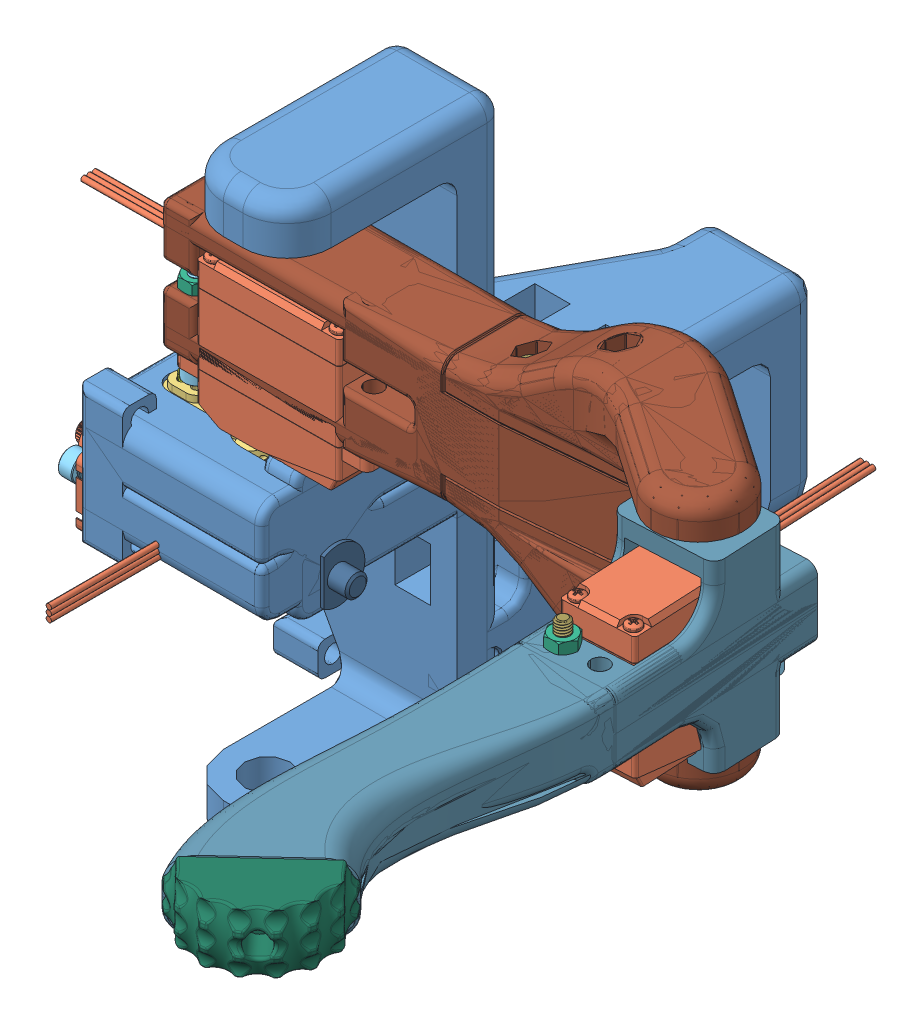
SolidWorks assembly Jambe_gauche, configuration Default. Lengths in mm.
Overall size (226.75 105.95 225.72).
41 component instances, 15 part files, 4 mates.
Components (placement in the parent):
- Hanche-1: Hanche [Default] at origin size (77.1 102.9 99.1)
  - Hanche_V3-1: Hanche_V3 [Default] at origin size (51.8 165 157.2)
  - Servo_DS3225MG-1: Servo_DS3225MG [Default] at (-27.6 -10.2 0) x (0 0 -1) z (-1 0 0) size (87.25 20.4 45.91)
  - Servo_helice-1: Servo_helice [Défaut] at (24 10 0) x (-1 0 0) z (0 -1 0) size (35.39 15.87 6)
  - bearing_535198-1: bearing_535198 [Défaut] at (24 72.6322 0) x (-0.923922 0 -0.382581) z (-0.382581 0 0.923922) size (13.87 4.75 13.87)
  - M4x25mm-1: M4x25mm [91290A176] at (12 -5.2 14.8) x (0 -0.924225 -0.381849) z (1 0 0) size (7 7 29.41)
  - M4x25mm-2: M4x25mm [91290A176] at (12 -15.2 -34.8) x (0 -0.924225 -0.381849) z (1 0 0) size (7 7 29.41)
  - M4_nut-1: M4_nut [90592A090] at (4.3 -15.2 -34.8) x (0 0.866025 0.5) z (0 -0.5 0.866025) size (7 3.75 8.08)
  - M4_nut-2: M4_nut [90592A090] at (4.3 -5.2 14.8) x (0 -0.866025 0.5) z (0 0.5 0.866025) size (7 3.75 8.08)
  - M2x16mm-1: M2x16mm [91290A047] at (24 19 0) x (1 0 0) z (0 1 0) size (3.8 3.8 18.16)
  - M2x16mm-2: M2x16mm [91290A047] at (0 18.4 0) x (1 0 0) z (0 1 0) size (3.8 3.8 18.16)
  - M3x30mm-1: M3x30mm [91290A171] at (29.5 33 -42.25) x (1 0 0) z (0 1 0) size (5.5 5.5 33.33)
  - M3x30mm-2: M3x30mm [91290A171] at (9.5 33 -42.25) x (1 0 0) z (0 1 0) size (5.5 5.5 33.33)
  - M3_nut-1: M3_nut [90592A085] at (29.5 26.2 -42.25) x (0.866025 0 -0.5) z (0.5 0 0.866025) size (5.5 2.79 6.35)
  - M3_nut-2: M3_nut [90592A085] at (9.5 26.2 -42.25) x (0.866025 0 -0.5) z (0.5 0 0.866025) size (5.5 2.79 6.35)
  - Cylinde_bearing-1: Cylinde_bearing [Default] at (37.5 -10.2 0) x (0 -1 0) z (1 0 0) size (15 11.5 12)
- Femur-1: Femur [Default] at (24 49.05 0) x (0 1 0) z (0.999976 0 -0.006973) size (73 46.33 202.15)
  - Femur_V3-1: Femur_V3 [Default] at origin size (73 46.33 172.05)
  - Servo_DS3225MG-1: Servo_DS3225MG [Default] at (-36.05 0 0) x (0 0 1) z (-1 0 0) size (87.25 20.4 45.91)
  - M4x25mm-1: M4x25mm [91290A176] at (3.55 5 -14.8) x (0 -0.070308 -0.997525) z (1 0 0) size (7 7 29.41)
  - M4x25mm-2: M4x25mm [91290A176] at (3.55 -5 34.8) x (0 -0.99819 0.060141) z (1 0 0) size (7 7 29.41)
  - M4_nut-1: M4_nut [90592A090] at (-1.65 5 -14.8) x (0 0.5 0.866025) z (0 -0.866025 0.5) size (7 3.75 8.08)
  - M4_nut-2: M4_nut [90592A090] at (-1.65 -5 34.8) x (0 1 0) z (0 0 1) size (7 3.75 8.08)
  - M4x30mm-1: M4x30mm [91290A180] at (-17 -2.3 71.7972) x (0 0 1) z (-1 0 0) size (7 7 34.38)
  - M4x30mm-2: M4x30mm [91290A180] at (-17 -2.3 96.7972) x (0 0 1) z (-1 0 0) size (7 7 34.38)
  - M4_nut-3: M4_nut [90592A090] at (-14.6 -2.3 71.7972) x (0 0.5 0.866025) z (0 -0.866025 0.5) size (7 3.75 8.08)
  - M4_nut-4: M4_nut [90592A090] at (-14.6 -2.3 96.7972) x (0 1 0) z (0 0 1) size (7 3.75 8.08)
  - Servo_helice-1: Servo_helice [Défaut] at (-32.5 18.86 139.55) x (0 -0.573576 -0.819152) z (-1 0 0) size (35.39 15.87 6)
  - M2_8-1: M2_8 [91292A012] at (-25.5 5.0942 119.8904) x (0 0.030232 -0.999543) z (1 0 0) size (4.5 4.5 10.65)
  - M2_8-2: M2_8 [91292A012] at (-25.5 18.86 139.55) x (0 0.030232 -0.999543) z (1 0 0) size (4.5 4.5 10.65)
  - Cylinde_bearing-1: Cylinde_bearing [Default] at (12.75 0 0) x (0 0 1) z (1 0 0) size (15 11.5 12)
- Tibia-1: Tibia [Default] at (163.6781 57.4324 17.8865) x (0.047809 0 0.998857) z (0.998857 0 -0.047809) size (207.93 61.42 52.63)
  - Tibia_V3-1: Tibia_V3 [Default] at origin size (162.76 52 39.97)
  - Embout_TPE_V3-1: Embout_TPE_V3 [Default] at (129.9518 8.3 0.0575) x (0 -1 0) z (0.642788 0 -0.766044) size (17.12 19.75 39.79)
  - Servo_DS3225MG-1: Servo_DS3225MG [Default] at (0 37.8 0) x (1 0 0) z (0 1 0) size (87.25 20.4 45.91)
  - bearing_535198-1: bearing_535198 [Défaut] at (0 -12.3678 0) x (0.863205 0 0.504854) z (0.504854 0 -0.863205) size (13.87 4.75 13.87)
  - Cylinde_bearing-1: Cylinde_bearing [Default] at (0 -11.6176 0) x (-0.99451 0 0.104639) z (0 -1 0) size (15 11.5 12)
  - M4x25mm-1: M4x25mm [91290A176] at (-14.8 -1.8 5) x (-0.837169 0 -0.546944) z (0 -1 0) size (7 7 29.41)
  - M4x30mm-1: M4x30mm [91290A180] at (34.8 -6.8 -5) x (-0.837169 0 -0.546944) z (0 -1 0) size (7 7 34.38)
  - M4_nut-1: M4_nut [90592A090] at (-14.8 3.4 5) x (0.5 0 0.866025) z (-0.866025 0 0.5) size (7 3.75 8.08)
  - M4_nut-2: M4_nut [90592A090] at (34.8 -1.6 -5) size (7 3.75 8.08)
Mates (geometry in assembly coordinates):
- Concentric1: concentric aligned: cylinder of Hanche-1/bearing_535198-1 through (24 72.6322 0) axis (0 -1 0) radius 3.175; cylinder of Femur-1/Femur_V3-1 through (24 59.8 0) axis (0 -1 0) radius 3.15
- Distance1: distance = 1 mm anti-aligned: plane of Hanche-1/Servo_helice-1 through (24 16 0) normal (0 1 0); plane of Femur-1/Servo_DS3225MG-1 through (24 17 0) normal (0 -1 0)
- Concentric2: concentric aligned: cylinder of Femur-1/Femur_V3-1 through (163.6781 83.05 17.8865) axis (0 -1 0) radius 3.15; cylinder of Tibia-1/Cylinde_bearing-1 through (163.6781 81.05 17.8865) axis (0 -1 0) radius 3.1
- Coincident4: coincident anti-aligned: plane of Femur-1/Femur_V3-1 through (176.9382 75.55 126.8518) normal (0 -1 0); plane of Tibia-1/Cylinde_bearing-1 through (163.6781 75.55 17.8865) normal (0 1 0)
